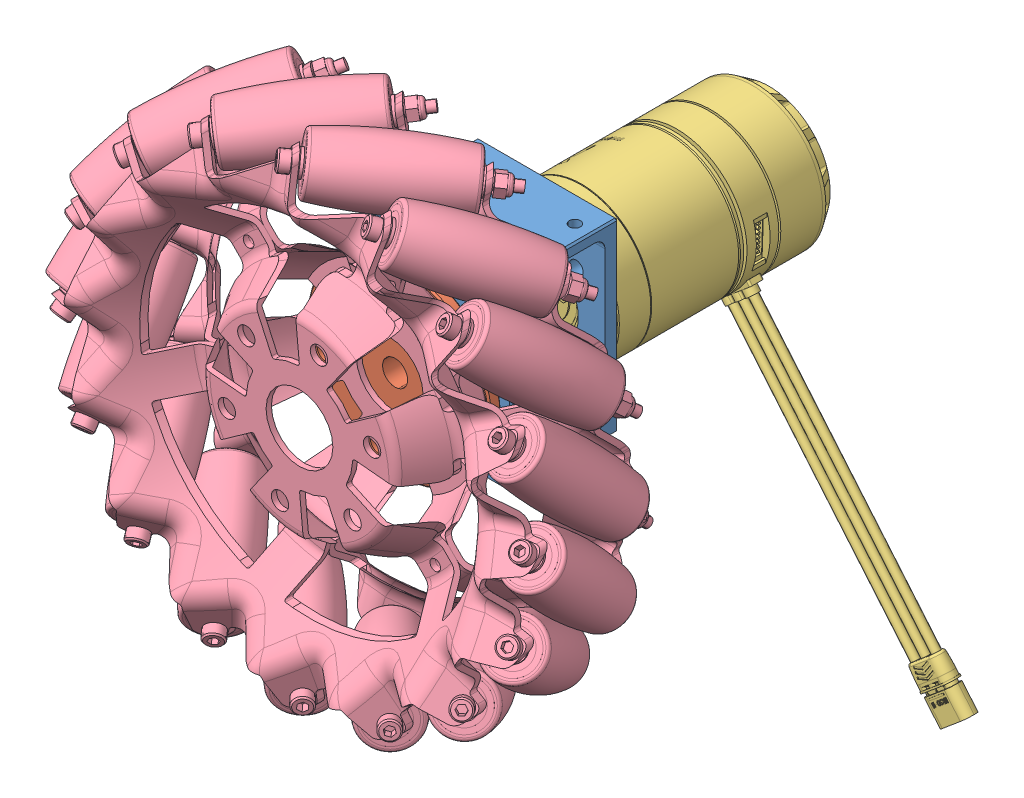
SolidWorks assembly 麦轮总装左轮, configuration 默认. Lengths in mm.
Overall size (230.42 230.42 154.75).
5 component instances, 4 part files, 3 mates.
Components (placement in the parent):
- 3508-1: 3508 [Default] at (43.0796 -3.0277 90.2458) size (124.33 157.68 116.9)
  - 电机座Z80123-1: 电机座Z80123 [默认] at (-77.6885 26.4734 96.0875) size (42 55.4 32)
  - 电机连轴Z80123-1: 电机连轴Z80123 [默认] at (-77.6885 26.4734 125.8875) x (0.707107 -0.707107 0) z (0.707107 0.707107 0) size (55 37.5 55)
  - M3508直流无刷减速电机-2: M3508直流无刷减速电机 [默认] at (-69.0293 10.2886 -6.3535) x (0.923508 0.383579 0) z (0 0 1) size (63.71 141 98.4)
- 麦轮镂空（左）-1: 麦轮镂空（左） [默认] at (-104.2541 -78.9214 138.5246) x (-0.707107 0.707107 0) z (0.707107 0.707107 0) size (178.66 47.46 178.66)
Mates (geometry in assembly coordinates):
- 重合1: coincident anti-aligned: plane of 3508-1/电机连轴Z80123-1 through (-34.6089 23.4456 216.1333) normal (0 0 1); plane of 麦轮镂空（左）-1 through (-30.1604 -21.7201 216.1333) normal (0 0 -1)
- 同心1: concentric anti-aligned: cylinder of 3508-1/电机连轴Z80123-1 through (-34.6089 23.4456 216.1333) axis (0 0 -1) radius 3.75; cylinder of 麦轮镂空（左）-1 through (-34.6089 23.4456 215.9721) axis (0 0 1) radius 10
- 同心2: concentric aligned: cylinder of 3508-1/电机连轴Z80123-1 through (-56.3422 17.6222 205.1333) axis (0 0 1) radius 2.6; cylinder of 麦轮镂空（左）-1 through (-56.3422 17.6222 242.9723) axis (0 0 1) radius 2.6
